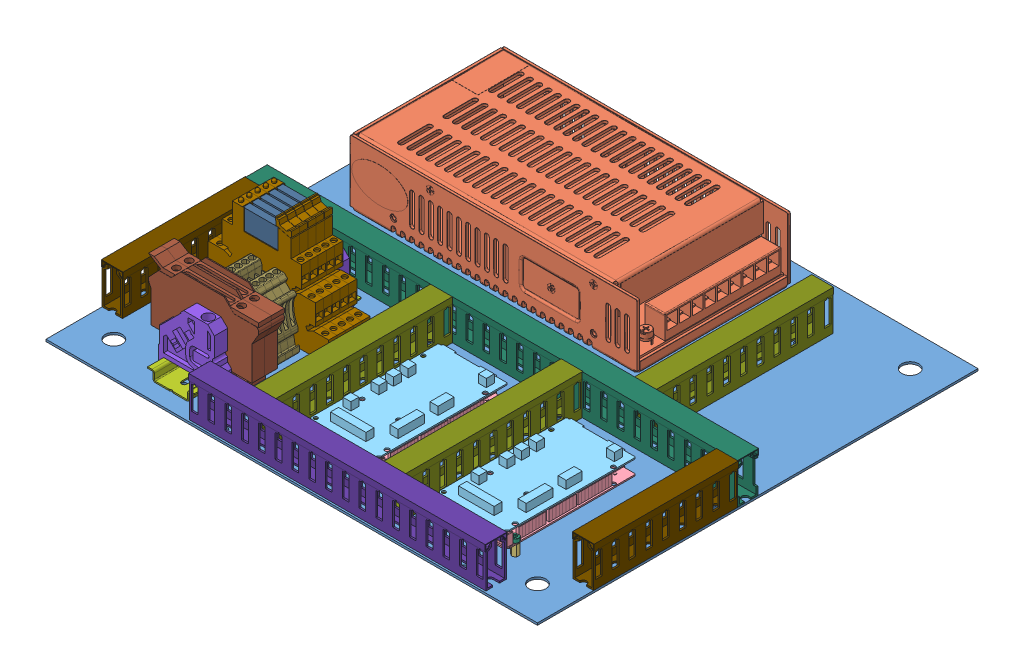
SolidWorks assembly elc component panel, configuration Default. Lengths in mm.
Overall size (369.37 194.67 371.79).
68 component instances, 18 part files, 51 mates.
Components (placement in the parent):
- elc plate-1: elc plate [Default] at (226.2293 207.4053 266.8793) size (368.3 1.59 330.2)
- power supply with standoffs-1: power supply with standoffs [Default] at (35.6304 133.9192 294.786) x (0 0 -1) z (1 0 0) size (115.2 58.27 215)
  - __-1: __ [По умолчанию] at (110.1067 83.0736 152.0488) size (115.2 50.11 215)
  - 95783A055_NYLON 6 6 MALE-FEMALE THREADED HEX STANDOFF-1: 95783A055_NYLON 6 6 MALE-FEMALE THREADED HEX STANDOFF [95783A055] at (85.1067 81.4236 77.0488) x (0 1 0) z (0 0 1) size (13.03 5.2 4.5)
  - 95783A055_NYLON 6 6 MALE-FEMALE THREADED HEX STANDOFF-2: 95783A055_NYLON 6 6 MALE-FEMALE THREADED HEX STANDOFF [95783A055] at (135.1067 81.4236 77.0488) x (0 1 0) z (-0.939028 0 -0.343839) size (13.03 5.2 4.5)
  - 95783A055_NYLON 6 6 MALE-FEMALE THREADED HEX STANDOFF-3: 95783A055_NYLON 6 6 MALE-FEMALE THREADED HEX STANDOFF [95783A055] at (135.1067 81.4236 227.0488) x (0 1 0) z (-0.996262 0 -0.086381) size (13.03 5.2 4.5)
  - 95783A055_NYLON 6 6 MALE-FEMALE THREADED HEX STANDOFF-4: 95783A055_NYLON 6 6 MALE-FEMALE THREADED HEX STANDOFF [95783A055] at (85.1067 81.4236 227.0488) x (0 1 0) z (-0.990494 0 -0.137554) size (13.03 5.2 4.5)
- arduino board assembly-1: arduino board assembly [Default] at (260.6228 173.6976 405.5467) x (0 0 -1) z (1 0 0) size (100 30.86 52.88)
  - ArduinoMega2560 CORRECTED-1: ArduinoMega2560 CORRECTED [Default] at (48.9673 43.2952 72.715) size (100 11.65 51.63)
  - breakout board-1: breakout board [Default] at (48.9673 54.2952 72.715) size (100 7 51.63)
  - 95783A055_NYLON 6 6 MALE-FEMALE THREADED HEX STANDOFF-1: 95783A055_NYLON 6 6 MALE-FEMALE THREADED HEX STANDOFF [95783A055] at (84.2031 36.9452 49.5995) x (0 -1 0) z (0 0 1) size (13.03 5.2 4.5)
  - 95783A055_NYLON 6 6 MALE-FEMALE THREADED HEX STANDOFF-2: 95783A055_NYLON 6 6 MALE-FEMALE THREADED HEX STANDOFF [95783A055] at (3.483 36.9452 49.7272) x (0 -1 0) z (0 0 1) size (13.03 5.2 4.5)
  - 95783A055_NYLON 6 6 MALE-FEMALE THREADED HEX STANDOFF-3: 95783A055_NYLON 6 6 MALE-FEMALE THREADED HEX STANDOFF [95783A055] at (9.6911 36.9452 96.9805) x (0 -1 0) z (0 0 1) size (13.03 5.2 4.5)
  - 91290A110_BLACK-OXIDE CLASS 12.9 SOCKET HEAD CAP SCREW-1: 91290A110_BLACK-OXIDE CLASS 12.9 SOCKET HEAD CAP SCREW [91290A110] at (9.6911 39.2952 96.9805) x (1 0 0) z (0 -1 0) size (5.5 5.5 8.18)
  - 91290A110_BLACK-OXIDE CLASS 12.9 SOCKET HEAD CAP SCREW-2: 91290A110_BLACK-OXIDE CLASS 12.9 SOCKET HEAD CAP SCREW [91290A110] at (84.2031 39.2952 49.5995) x (1 0 0) z (0 -1 0) size (5.5 5.5 8.18)
  - 91290A110_BLACK-OXIDE CLASS 12.9 SOCKET HEAD CAP SCREW-3: 91290A110_BLACK-OXIDE CLASS 12.9 SOCKET HEAD CAP SCREW [91290A110] at (3.483 39.2952 49.7272) x (1 0 0) z (0 -1 0) size (5.5 5.5 8.18)
- din rail assmbly-1: din rail assmbly [Default] at (226.6874 101.8607 473.572) x (-1 0 0) z (0 0 -1) size (189.42 194.67 179.29)
  - DIN 59_0-1: DIN 59_0 [00] at (103.6081 107.1321 54.2926) size (35 7.5 125)
  - SEIMENS 8WA1 808 DIN RAIL END RETAINER-1: SEIMENS 8WA1 808 DIN RAIL END RETAINER [Default] at (102.6081 107.6321 71.2884) size (45 44.95 10)
  - SEIMENS 8WA1 808 DIN RAIL END RETAINER-3: SEIMENS 8WA1 808 DIN RAIL END RETAINER [Default] at (102.6081 107.6321 162.4924) size (45 44.95 10)
  - 3812830-8: 3812830 [Default] at (102.7638 140.3713 56.6988) x (0 0 -1) z (1 0 0) size (6.2 76.69 90.31)
    - 3812830A-1: 3812830A [Default] at (-75.9936 -29.2392 18.3443) size (6.2 76.69 90.31)
    - 3812830B-1: 3812830B [Default] at (-75.3936 25.9608 19.6) size (5 19.3 28)
  - 3812830-9: 3812830 [Default] at (102.7638 140.3713 62.8988) x (0 0 -1) z (1 0 0) size (6.2 76.69 90.31)
    - 3812830A-1: 3812830A [Default] at (-75.9936 -29.2392 18.3443) size (6.2 76.69 90.31)
    - 3812830B-1: 3812830B [Default] at (-75.3936 25.9608 19.6) size (5 19.3 28)
  - 3812830-10: 3812830 [Default] at (102.7638 140.3713 69.0988) x (0 0 -1) z (1 0 0) size (6.2 76.69 90.31)
    - 3812830A-1: 3812830A [Default] at (-75.9936 -29.2392 18.3443) size (6.2 76.69 90.31)
    - 3812830B-1: 3812830B [Default] at (-75.3936 25.9608 19.6) size (5 19.3 28)
  - 3812830-11: 3812830 [Default] at (102.7638 140.3713 75.2988) x (0 0 -1) z (1 0 0) size (6.2 76.69 90.31)
    - 3812830A-1: 3812830A [Default] at (-75.9936 -29.2392 18.3443) size (6.2 76.69 90.31)
    - 3812830B-1: 3812830B [Default] at (-75.3936 25.9608 19.6) size (5 19.3 28)
  - 3812830-12: 3812830 [Default] at (102.7638 140.3713 81.4988) x (0 0 -1) z (1 0 0) size (6.2 76.69 90.31)
    - 3812830A-1: 3812830A [Default] at (-75.9936 -29.2392 18.3443) size (6.2 76.69 90.31)
    - 3812830B-1: 3812830B [Default] at (-75.3936 25.9608 19.6) size (5 19.3 28)
  - Din fuse-1: Din fuse [Default] at (59.9389 109.5521 90.7664) size (82.55 57.15 9.65)
  - Din fuse-2: Din fuse [Default] at (59.9389 109.5521 81.1144) size (82.55 57.15 9.65)
  - dinrail_Terminal-11: dinrail_Terminal [Default] at (121.1081 114.6321 95.5924) size (48 46.85 5.15)
  - dinrail_Terminal-12: dinrail_Terminal [Default] at (121.1081 114.6321 100.7424) size (48 46.85 5.15)
  - dinrail_Terminal-13: dinrail_Terminal [Default] at (121.1081 114.6321 111.0424) size (48 46.85 5.15)
  - dinrail_Terminal-16: dinrail_Terminal [Default] at (121.1081 114.6321 105.8924) size (48 46.85 5.15)
  - dinrail_Terminal-17: dinrail_Terminal [Default] at (121.1081 114.6321 116.1924) size (48 46.85 5.15)
  - dinrail_Terminal-18: dinrail_Terminal [Default] at (121.1081 114.6321 121.3424) size (48 46.85 5.15)
- arduino board assembly-2: arduino board assembly [Default] at (164.5922 173.6976 405.5467) x (0 0 -1) z (1 0 0) size (100 30.86 52.88)
  - ArduinoMega2560 CORRECTED-1: ArduinoMega2560 CORRECTED [Default] at (48.9673 43.2952 72.715) size (100 11.65 51.63)
  - breakout board-1: breakout board [Default] at (48.9673 54.2952 72.715) size (100 7 51.63)
  - 95783A055_NYLON 6 6 MALE-FEMALE THREADED HEX STANDOFF-1: 95783A055_NYLON 6 6 MALE-FEMALE THREADED HEX STANDOFF [95783A055] at (84.2031 36.9452 49.5995) x (0 -1 0) z (0 0 1) size (13.03 5.2 4.5)
  - 95783A055_NYLON 6 6 MALE-FEMALE THREADED HEX STANDOFF-2: 95783A055_NYLON 6 6 MALE-FEMALE THREADED HEX STANDOFF [95783A055] at (3.483 36.9452 49.7272) x (0 -1 0) z (0 0 1) size (13.03 5.2 4.5)
  - 95783A055_NYLON 6 6 MALE-FEMALE THREADED HEX STANDOFF-3: 95783A055_NYLON 6 6 MALE-FEMALE THREADED HEX STANDOFF [95783A055] at (9.6911 36.9452 96.9805) x (0 -1 0) z (0 0 1) size (13.03 5.2 4.5)
  - 91290A110_BLACK-OXIDE CLASS 12.9 SOCKET HEAD CAP SCREW-1: 91290A110_BLACK-OXIDE CLASS 12.9 SOCKET HEAD CAP SCREW [91290A110] at (9.6911 39.2952 96.9805) x (1 0 0) z (0 -1 0) size (5.5 5.5 8.18)
  - 91290A110_BLACK-OXIDE CLASS 12.9 SOCKET HEAD CAP SCREW-2: 91290A110_BLACK-OXIDE CLASS 12.9 SOCKET HEAD CAP SCREW [91290A110] at (84.2031 39.2952 49.5995) x (1 0 0) z (0 -1 0) size (5.5 5.5 8.18)
  - 91290A110_BLACK-OXIDE CLASS 12.9 SOCKET HEAD CAP SCREW-3: 91290A110_BLACK-OXIDE CLASS 12.9 SOCKET HEAD CAP SCREW [91290A110] at (3.483 39.2952 49.7272) x (1 0 0) z (0 -1 0) size (5.5 5.5 8.18)
- 92497A200_ZINC YELLOW-CHROMATE PLATED STEEL HEX NUT-1: 92497A200_ZINC YELLOW-CHROMATE PLATED STEEL HEX NUT [92497A200] at (214.3194 206.2053 402.0637) x (1 0 0) z (0 1 0) size (5.5 6.35 2.78)
- 92497A200_ZINC YELLOW-CHROMATE PLATED STEEL HEX NUT-2: 92497A200_ZINC YELLOW-CHROMATE PLATED STEEL HEX NUT [92497A200] at (214.1917 206.2053 321.3436) x (1 0 0) z (0 1 0) size (5.5 6.35 2.78)
- 92497A200_ZINC YELLOW-CHROMATE PLATED STEEL HEX NUT-3: 92497A200_ZINC YELLOW-CHROMATE PLATED STEEL HEX NUT [92497A200] at (261.5727 206.2053 395.8556) x (1 0 0) z (0 1 0) size (5.5 6.35 2.78)
- 92497A200_ZINC YELLOW-CHROMATE PLATED STEEL HEX NUT-4: 92497A200_ZINC YELLOW-CHROMATE PLATED STEEL HEX NUT [92497A200] at (310.3501 206.2053 402.0637) x (1 0 0) z (0 1 0) size (5.5 6.35 2.78)
- 92497A200_ZINC YELLOW-CHROMATE PLATED STEEL HEX NUT-5: 92497A200_ZINC YELLOW-CHROMATE PLATED STEEL HEX NUT [92497A200] at (310.2224 206.2053 321.3436) x (1 0 0) z (0 1 0) size (5.5 6.35 2.78)
- 92497A200_ZINC YELLOW-CHROMATE PLATED STEEL HEX NUT-6: 92497A200_ZINC YELLOW-CHROMATE PLATED STEEL HEX NUT [92497A200] at (357.6034 206.2053 395.8556) x (1 0 0) z (0 1 0) size (5.5 6.35 2.78)
- 92095A177_18-8 SS BUTTON-HEAD SOCKET CAP SCREW-1: 92095A177_18-8 SS BUTTON-HEAD SOCKET CAP SCREW [92095A177] at (262.6793 205.7553 159.6793) x (1 0 0) z (0 -1 0) size (5.7 5.7 6.94)
- 92095A177_18-8 SS BUTTON-HEAD SOCKET CAP SCREW-3: 92095A177_18-8 SS BUTTON-HEAD SOCKET CAP SCREW [92095A177] at (112.6793 205.7553 159.6793) x (1 0 0) z (0 -1 0) size (5.7 5.7 6.94)
- 92095A177_18-8 SS BUTTON-HEAD SOCKET CAP SCREW-4: 92095A177_18-8 SS BUTTON-HEAD SOCKET CAP SCREW [92095A177] at (112.6793 205.7553 209.6793) x (1 0 0) z (0 -1 0) size (5.7 5.7 6.94)
- small panduit 1-2: small panduit 1 [Default] at (435.7793 210.2628 274.3593) size (368.3 30.38 16.31)
- small panduit 4-6: small panduit 4 [Default] at (286.3538 210.2628 21.6293) x (0 0 -1) z (1 0 0) size (133.35 30.38 16.31)
- small panduit 4-7: small panduit 4 [Default] at (188.9955 210.2628 21.6293) x (0 0 -1) z (1 0 0) size (133.35 30.38 16.31)
- small panduit 4-8: small panduit 4 [Default] at (325.6017 210.2628 527.0893) x (0 0 1) z (-1 0 0) size (133.35 30.38 16.31)
- small panduit 3-2: small panduit 3 [Default] at (541.8293 210.2628 422.9493) size (222.25 30.38 16.31)
- small panduit 2-10: small panduit 2 [Default] at (49.6993 210.2628 -3.7707) x (0 0 -1) z (1 0 0) size (107.95 30.38 16.31)
- small panduit 2-11: small panduit 2 [Default] at (402.7593 210.2628 -3.7707) x (0 0 -1) z (1 0 0) size (107.95 30.38 16.31)
Mates (geometry in assembly coordinates):
- Coincident4: coincident: plane of elc plate-1 through (226.2293 208.9928 266.8793) normal (0 1 0); plane of arduino board assembly-1/95783A055_NYLON 6 6 MALE-FEMALE THREADED HEX STANDOFF-1 through (310.2224 208.9928 318.7455) normal (0 -1 0)
- Coincident5: coincident: plane of elc plate-1 through (226.2293 208.9928 266.8793) normal (0 1 0); plane of din rail assmbly-1/DIN 59_0-1 through (136.5793 208.9928 294.2793) normal (0 -1 0)
- Parallel2: parallel: plane of elc plate-1 through (410.3793 208.9928 101.7793) normal (1 0 0); plane of arduino board assembly-1/ArduinoMega2560 CORRECTED-1 through (359.5793 207.9928 308.1039) normal (1 0 0)
- Coincident8: coincident: plane of elc plate-1 through (226.2293 208.9928 266.8793) normal (0 1 0); plane of arduino board assembly-2/95783A055_NYLON 6 6 MALE-FEMALE THREADED HEX STANDOFF-3 through (261.5727 208.9928 393.2575) normal (0 -1 0)
- Parallel3: parallel: plane of arduino board assembly-1/breakout board-1 through (307.9466 218.9928 306.5793) normal (-1 0 0); line of arduino board assembly-2/ArduinoMega2560 CORRECTED-1 through (263.5486 216.9928 308.1039) axis (0 0 1)
- Coincident28: coincident: plane of arduino board assembly-1/ArduinoMega2560 CORRECTED-1 through (350.3515 225.9928 306.5793) normal (0 0 -1); line of arduino board assembly-2/ArduinoMega2560 CORRECTED-1 through (242.4708 225.9928 306.5793) axis (1 0 0)
- Coincident36: coincident: plane of elc plate-1 through (226.2293 207.4053 266.8793) normal (0 -1 0); plane of 92497A200_ZINC YELLOW-CHROMATE PLATED STEEL HEX NUT-1 through (211.5694 207.4053 400.476) normal (0 1 0)
- Concentric1: concentric: cylinder of arduino board assembly-2/91290A110_BLACK-OXIDE CLASS 12.9 SOCKET HEAD CAP SCREW-3 through (214.3194 220.9928 402.0637) axis (0 -1 0) radius 2.75; circle of 92497A200_ZINC YELLOW-CHROMATE PLATED STEEL HEX NUT-1
- Coincident37: coincident: plane of elc plate-1 through (226.2293 207.4053 266.8793) normal (0 -1 0); plane of 92497A200_ZINC YELLOW-CHROMATE PLATED STEEL HEX NUT-3 through (258.8227 207.4053 394.2679) normal (0 1 0)
- Concentric2: concentric: cylinder of arduino board assembly-2/91290A110_BLACK-OXIDE CLASS 12.9 SOCKET HEAD CAP SCREW-1 through (261.5727 220.9928 395.8556) axis (0 -1 0) radius 2.75; circle of 92497A200_ZINC YELLOW-CHROMATE PLATED STEEL HEX NUT-3
- Coincident38: coincident: plane of elc plate-1 through (226.2293 207.4053 266.8793) normal (0 -1 0); plane of 92497A200_ZINC YELLOW-CHROMATE PLATED STEEL HEX NUT-2 through (211.4417 207.4053 319.7559) normal (0 1 0)
- Concentric3: concentric: cylinder of elc plate-1 through (214.1917 208.9938 321.3436) axis (0 -1 0) radius 1.665; circle of 92497A200_ZINC YELLOW-CHROMATE PLATED STEEL HEX NUT-2
- Coincident39: coincident: plane of elc plate-1 through (226.2293 207.4053 266.8793) normal (0 -1 0); plane of 92497A200_ZINC YELLOW-CHROMATE PLATED STEEL HEX NUT-4 through (307.6001 207.4053 400.476) normal (0 1 0)
- Concentric4: concentric: cylinder of elc plate-1 through (310.3501 208.9938 402.0637) axis (0 -1 0) radius 1.665; circle of 92497A200_ZINC YELLOW-CHROMATE PLATED STEEL HEX NUT-4
- Coincident40: coincident: plane of elc plate-1 through (226.2293 207.4053 266.8793) normal (0 -1 0); plane of 92497A200_ZINC YELLOW-CHROMATE PLATED STEEL HEX NUT-6 through (354.8534 207.4053 394.2679) normal (0 1 0)
- Concentric5: concentric: cylinder of elc plate-1 through (357.6034 208.9938 395.8556) axis (0 -1 0) radius 1.665; circle of 92497A200_ZINC YELLOW-CHROMATE PLATED STEEL HEX NUT-6
- Coincident41: coincident: plane of elc plate-1 through (226.2293 207.4053 266.8793) normal (0 -1 0); plane of 92497A200_ZINC YELLOW-CHROMATE PLATED STEEL HEX NUT-5 through (307.4724 207.4053 319.7559) normal (0 1 0)
- Concentric6: concentric: cylinder of elc plate-1 through (310.2224 208.9938 321.3436) axis (0 -1 0) radius 1.665; circle of 92497A200_ZINC YELLOW-CHROMATE PLATED STEEL HEX NUT-5
- Coincident43: coincident: plane of elc plate-1 through (226.2293 207.4053 266.8793) normal (0 -1 0); plane of 92095A177_18-8 SS BUTTON-HEAD SOCKET CAP SCREW-1 through (262.6793 207.4053 156.8293) normal (0 1 0)
- Concentric8: concentric: cylinder of elc plate-1 through (262.6793 207.4043 159.6793) axis (0 1 0) radius 1.665; cylinder of 92095A177_18-8 SS BUTTON-HEAD SOCKET CAP SCREW-1 through (262.6793 205.7553 159.6793) axis (0 -1 0) radius 2.85
- Coincident44: coincident: plane of elc plate-1 through (226.2293 207.4053 266.8793) normal (0 -1 0); plane of 92095A177_18-8 SS BUTTON-HEAD SOCKET CAP SCREW-4 through (112.6793 207.4053 206.8293) normal (0 1 0)
- Concentric9: concentric: cylinder of elc plate-1 through (112.6793 207.4043 209.6793) axis (0 1 0) radius 1.665; cylinder of 92095A177_18-8 SS BUTTON-HEAD SOCKET CAP SCREW-4 through (112.6793 205.7553 209.6793) axis (0 -1 0) radius 2.85
- Coincident45: coincident: plane of elc plate-1 through (226.2293 207.4053 266.8793) normal (0 -1 0); plane of 92095A177_18-8 SS BUTTON-HEAD SOCKET CAP SCREW-3 through (112.6793 207.4053 156.8293) normal (0 1 0)
- Concentric10: concentric: cylinder of elc plate-1 through (112.6793 207.4043 159.6793) axis (0 1 0) radius 1.665; cylinder of 92095A177_18-8 SS BUTTON-HEAD SOCKET CAP SCREW-3 through (112.6793 205.7553 159.6793) axis (0 -1 0) radius 2.85
- Coincident62: coincident: plane of elc plate-1 through (226.2293 208.9928 266.8793) normal (0 1 0); plane of power supply with standoffs-1/95783A055_NYLON 6 6 MALE-FEMALE THREADED HEX STANDOFF-1 through (112.6793 208.9928 212.2774) normal (0 -1 0)
- Distance1: distance = 38.1 mm: plane of power supply with standoffs-1/__-1 through (80.1793 265.9928 184.6793) normal (-1 0 0); plane of elc plate-1 through (42.0793 208.9928 101.7793) normal (-1 0 0)
- Distance2: distance = 25.4 mm: plane of power supply with standoffs-1/__-1 through (80.1793 218.9928 127.1793) normal (0 0 -1); plane of elc plate-1 through (42.0793 208.9928 101.7793) normal (0 0 -1)
- Parallel4: parallel: line of elc plate-1 through (410.3793 207.4053 101.7793) axis (-1 0 0); plane of din rail assmbly-1/DIN 59_0-1 through (109.5793 209.9928 294.2793) normal (0 0 -1)
- Distance3: distance = 50.8 mm: plane of arduino board assembly-1/ArduinoMega2560 CORRECTED-1 through (359.5793 207.9928 308.1039) normal (1 0 0); plane of elc plate-1 through (410.3793 208.9928 101.7793) normal (1 0 0)
- Parallel5: parallel: plane of din rail assmbly-1/DIN 59_0-1 through (109.5793 216.4928 419.2793) normal (0 0 1); plane of arduino board assembly-2/ArduinoMega2560 CORRECTED-1 through (263.8072 217.9928 406.5793) normal (0 0 1)
- Distance4: distance = 12.7 mm: plane of din rail assmbly-1/DIN 59_0-1 through (136.5793 216.4928 419.2793) normal (0 0 1); plane of elc plate-1 through (42.0793 208.9928 431.9793) normal (0 0 1)
- Distance5: distance = 63.5 mm: plane of din rail assmbly-1/DIN 59_0-1 through (105.5793 216.4928 419.2793) normal (-1 0 0); plane of elc plate-1 through (42.0793 208.9928 101.7793) normal (-1 0 0)
- Distance6: distance = 25.4 mm: plane of arduino board assembly-1/ArduinoMega2560 CORRECTED-1 through (359.8379 217.9928 406.5793) normal (0 0 1); plane of elc plate-1 through (42.0793 208.9928 431.9793) normal (0 0 1)
- Coincident71: coincident: plane of elc plate-1 through (226.2293 208.9928 266.8793) normal (0 1 0); plane of small panduit 1-2 through (829.4793 208.9928 274.3593) normal (0 -1 0)
- Coincident72: coincident: plane of elc plate-1 through (410.3793 208.9928 101.7793) normal (1 0 0); plane of small panduit 1-2 through (410.3793 208.9928 266.2059) normal (1 0 0)
- Coincident73: coincident: plane of elc plate-1 through (226.2293 208.9928 266.8793) normal (0 1 0); plane of small panduit 4-6 through (286.3538 208.9928 -372.0707) normal (0 -1 0)
- Coincident74: coincident: plane of small panduit 1-2 through (829.4793 208.9928 281.9793) normal (0 0 1); plane of small panduit 4-6 through (278.2004 208.9928 281.9793) normal (0 0 -1)
- Distance7: distance = 150 mm: plane of small panduit 1-2 through (829.4793 208.9928 281.9793) normal (0 0 1); line of elc plate-1 through (42.0793 207.4053 431.9793) axis (1 0 0)
- Coincident76: coincident: plane of small panduit 1-2 through (829.4793 208.9928 281.9793) normal (0 0 1); plane of small panduit 4-7 through (180.8421 208.9928 281.9793) normal (0 0 -1)
- Coincident77: coincident: plane of elc plate-1 through (226.2293 208.9928 266.8793) normal (0 1 0); plane of small panduit 4-7 through (188.9955 208.9928 -372.0707) normal (0 -1 0)
- Coincident78: coincident: plane of small panduit 1-2 through (829.4793 208.9928 266.7393) normal (0 0 -1); plane of small panduit 4-8 through (333.7551 208.9928 266.7393) normal (0 0 1)
- Coincident79: coincident: plane of elc plate-1 through (226.2293 208.9928 266.8793) normal (0 1 0); plane of small panduit 4-8 through (325.6017 208.9928 920.7893) normal (0 -1 0)
- Coincident80: coincident: plane of elc plate-1 through (226.2293 208.9928 266.8793) normal (0 1 0); plane of small panduit 3-2 through (935.5293 208.9928 422.9493) normal (0 -1 0)
- Coincident81: coincident: plane of small panduit 4-6 through (286.3538 210.2628 415.3293) normal (0 0 1); plane of small panduit 3-2 through (935.5293 208.9928 415.3293) normal (0 0 -1)
- Distance8: distance = 40 mm: plane of small panduit 3-2 through (370.3793 208.9928 414.7959) normal (1 0 0); plane of elc plate-1 through (410.3793 208.9928 101.7793) normal (1 0 0)
- Coincident83: coincident: plane of small panduit 1-2 through (829.4793 208.9928 281.9793) normal (0 0 1); plane of small panduit 2-10 through (41.5459 208.9928 281.9793) normal (0 0 -1)
- Coincident84: coincident: plane of elc plate-1 through (226.2293 208.9928 266.8793) normal (0 1 0); plane of small panduit 2-10 through (49.6993 208.9928 -397.4707) normal (0 -1 0)
- Coincident85: coincident: plane of elc plate-1 through (42.0793 208.9928 101.7793) normal (-1 0 0); plane of small panduit 2-10 through (42.0793 208.9928 -397.4707) normal (-1 0 0)
- Coincident86: coincident: plane of small panduit 1-2 through (829.4793 208.9928 281.9793) normal (0 0 1); plane of small panduit 2-11 through (394.6059 208.9928 281.9793) normal (0 0 -1)
- Coincident87: coincident: plane of elc plate-1 through (226.2293 208.9928 266.8793) normal (0 1 0); plane of small panduit 2-11 through (402.7593 208.9928 -397.4707) normal (0 -1 0)
- Coincident88: coincident: line of elc plate-1 through (410.3793 207.4053 431.9793) axis (0 0 -1); plane of small panduit 2-11 through (410.3793 208.9928 -397.4707) normal (1 0 0)
